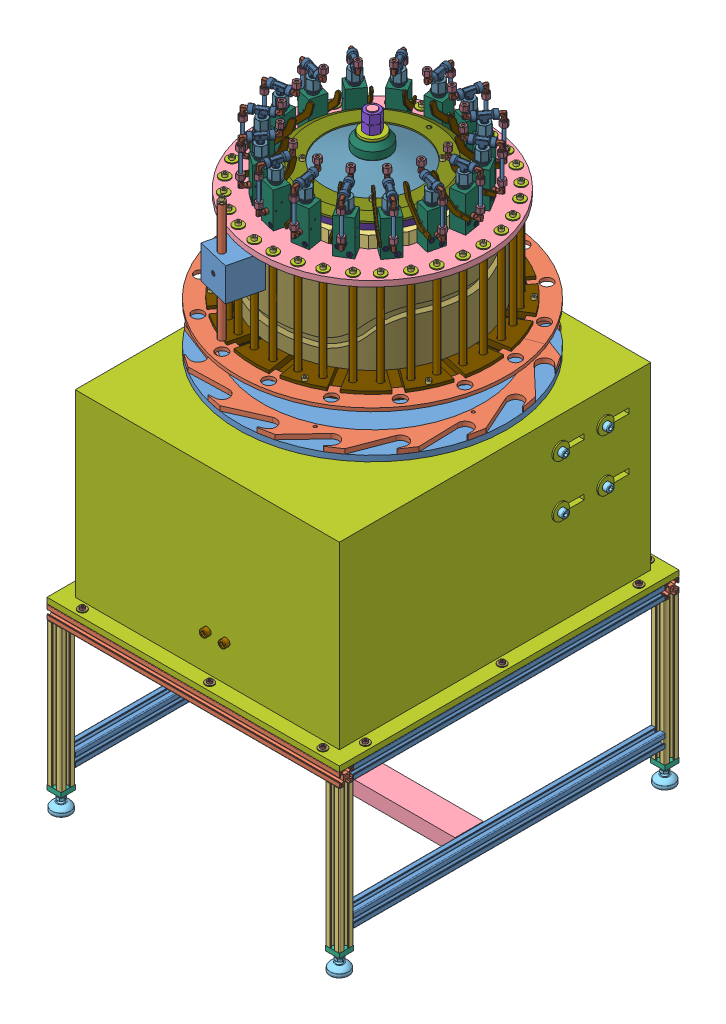
SolidWorks assembly Assieme_FINALE, configuration Default. Lengths in mm. (continued)
Components (placement in the parent): (continued)
- assieme parte rotante-2: assieme parte rotante [Default] at (-8.3038 623.9178 -528.0599) x (0 1 0) z (-0.913062 0 0.407822) size (749.63 778.63 778.63) (continued)
  - AssiemeValvola-14: AssiemeValvola [Default] at (515.3257 186.9093 437.1895) x (0 -0.991445 -0.130526) z (0 -0.130526 0.991445) size (90.26 138.63 38) (continued)
    - LevaValvola-1: LevaValvola [Default] at (-24.507 -86.571 -17) x (0.996193 0.087174 0) z (0 0 1) size (77.55 60.2 4)
    - Tubo-1: Tubo [Default] at (-30 -15.9665 0) x (1 0 0) z (0 -1 0) size (6 6 56.4)
  - AssiemeValvola-15: AssiemeValvola [Default] at (515.3257 182.5711 371.0008) x (0 -0.965926 0.258819) z (0 0.258819 0.965926) size (90.26 138.63 38)
    - RaccordoT-1: RaccordoT [Default] at origin size (43 29.75 16.5)
    - Raccordo a L-1: Raccordo a L [Default] at (-30 0 0) x (0 -1 0) z (0 0 -1) size (28.34 25.51 14.01)
      - 1809_06_10_01-1: 1809_06_10_01 [Default] at origin size (22.49 23 10)
      - 1809_06_10_02-1: 1809_06_10_02 [Default] at origin size (6.5 8.5 8.5)
      - 1809_06_10_03-1: 1809_06_10_03 [Default] at origin size (11.02 15.01 14.01)
    - Raccordo a L-2: Raccordo a L [Default] at (30 0 0) x (0 1 0) z (0 0 -1) size (28.34 25.51 14.01)
      - 1809_06_10_01-1: 1809_06_10_01 [Default] at origin size (22.49 23 10)
      - 1809_06_10_02-1: 1809_06_10_02 [Default] at origin size (6.5 8.5 8.5)
      - 1809_06_10_03-1: 1809_06_10_03 [Default] at origin size (11.02 15.01 14.01)
    - TappoChiusura-1: TappoChiusura [Default] at (0 -32 0) x (0 -1 0) z (0 0 1) size (38.28 26.74 26.74)
    - CorpoValvola-1: CorpoValvola [Default] at (-15 -115.2824 0) size (30 75 34)
    - Raccordo a L-3: Raccordo a L [Default] at (-30 -88.2824 0) x (0 1 0) z (0 0 1) size (28.34 25.51 14.01)
      - 1809_06_10_01-1: 1809_06_10_01 [Default] at origin size (22.49 23 10)
      - 1809_06_10_02-1: 1809_06_10_02 [Default] at origin size (6.5 8.5 8.5)
      - 1809_06_10_03-1: 1809_06_10_03 [Default] at origin size (11.02 15.01 14.01)
    - Spina_3x38-1: Spina_3x38 [Default] at (0 -68.2824 -21) x (-1 0 0) z (0 0 1) size (3 3 38)
    - Spina_3x38-2: Spina_3x38 [Default] at (-10 -80.2824 -21) x (0.996193 0.087174 0) z (0 0 1) size (3 3 38)
    - M5 40mm-3: M5 40mm [ISO 4762 M5 x 40 - 40N] at (-14.6 -108.7824 9) size (45 8.5 8.5)
    - M5 40mm-2: M5 40mm [ISO 4762 M5 x 40 - 40N] at (-14.6 -96.7824 -9) size (45 8.5 8.5)
    - LevaValvola-1: LevaValvola [Default] at (-24.507 -86.571 -17) x (0.996193 0.087174 0) z (0 0 1) size (77.55 60.2 4)
    - Tubo-1: Tubo [Default] at (-30 -15.9665 0) x (1 0 0) z (0 -1 0) size (6 6 56.4)
  - AssiemeValvola-16: AssiemeValvola [Default] at (515.3257 153.2338 311.5106) x (0 -0.793353 0.608761) z (0 0.608761 0.793353) size (90.26 138.63 38)
    - RaccordoT-1: RaccordoT [Default] at origin size (43 29.75 16.5)
    - Raccordo a L-1: Raccordo a L [Default] at (-30 0 0) x (0 -1 0) z (0 0 -1) size (28.34 25.51 14.01)
      - 1809_06_10_01-1: 1809_06_10_01 [Default] at origin size (22.49 23 10)
      - 1809_06_10_02-1: 1809_06_10_02 [Default] at origin size (6.5 8.5 8.5)
      - 1809_06_10_03-1: 1809_06_10_03 [Default] at origin size (11.02 15.01 14.01)
    - Raccordo a L-2: Raccordo a L [Default] at (30 0 0) x (0 1 0) z (0 0 -1) size (28.34 25.51 14.01)
      - 1809_06_10_01-1: 1809_06_10_01 [Default] at origin size (22.49 23 10)
      - 1809_06_10_02-1: 1809_06_10_02 [Default] at origin size (6.5 8.5 8.5)
      - 1809_06_10_03-1: 1809_06_10_03 [Default] at origin size (11.02 15.01 14.01)
    - TappoChiusura-1: TappoChiusura [Default] at (0 -32 0) x (0 -1 0) z (0 0 1) size (38.28 26.74 26.74)
    - CorpoValvola-1: CorpoValvola [Default] at (-15 -115.2824 0) size (30 75 34)
    - Raccordo a L-3: Raccordo a L [Default] at (-30 -88.2824 0) x (0 1 0) z (0 0 1) size (28.34 25.51 14.01)
      - 1809_06_10_01-1: 1809_06_10_01 [Default] at origin size (22.49 23 10)
      - 1809_06_10_02-1: 1809_06_10_02 [Default] at origin size (6.5 8.5 8.5)
      - 1809_06_10_03-1: 1809_06_10_03 [Default] at origin size (11.02 15.01 14.01)
    - Spina_3x38-1: Spina_3x38 [Default] at (0 -68.2824 -21) x (-1 0 0) z (0 0 1) size (3 3 38)
    - Spina_3x38-2: Spina_3x38 [Default] at (-10 -80.2824 -21) x (0.996193 0.087174 0) z (0 0 1) size (3 3 38)
    - M5 40mm-3: M5 40mm [ISO 4762 M5 x 40 - 40N] at (-14.6 -108.7824 9) size (45 8.5 8.5)
    - M5 40mm-2: M5 40mm [ISO 4762 M5 x 40 - 40N] at (-14.6 -96.7824 -9) size (45 8.5 8.5)
    - LevaValvola-1: LevaValvola [Default] at (-24.507 -86.571 -17) x (0.996193 0.087174 0) z (0 0 1) size (77.55 60.2 4)
    - Tubo-1: Tubo [Default] at (-30 -15.9665 0) x (1 0 0) z (0 -1 0) size (6 6 56.4)
  - Disco alimentazione guarnizione fi24.4-1: Disco alimentazione guarnizione fi24.4 [Default] at (198.0433 18.3637 415) x (0 0.065403 0.997859) z (-1 0 0) size (570 285 7.35)
  - Disco alimentazione guarnizione fi24.4-2: Disco alimentazione guarnizione fi24.4 [Default] at (198.0433 18.3637 415) x (0 -0.065403 -0.997859) z (-1 0 0) size (570 285 7.35)
  - m6 12mm-1: m6 12mm [ISO 4762 M6 x 12 - 12N] at (210.0433 200.6849 574.8914) x (-1 0 0) z (0 0.793353 -0.608761) size (18 10 10)
  - m6 12mm-7: m6 12mm [ISO 4762 M6 x 12 - 12N] at (210.0433 260.3445 399.1397) x (-1 0 0) z (0 0.793353 -0.608761) size (18 10 10)
  - m6 12mm-8: m6 12mm [ISO 4762 M6 x 12 - 12N] at (210.0433 96.3128 185.3694) x (-1 0 0) z (0 0.793353 -0.608761) size (18 10 10)
  - m6 12mm-9: m6 12mm [ISO 4762 M6 x 12 - 12N] at (210.0433 -59.5854 644.6306) x (-1 0 0) z (0 -0.793353 -0.608761) size (18 10 10)
  - m6 12mm-10: m6 12mm [ISO 4762 M6 x 12 - 12N] at (210.0433 -223.6171 430.8603) x (-1 0 0) z (0 -0.793353 -0.608761) size (18 10 10)
  - m6 12mm-11: m6 12mm [ISO 4762 M6 x 12 - 12N] at (210.0433 -163.9575 255.1086) x (-1 0 0) z (0 0.793353 -0.608761) size (18 10 10)
- assieme parte fissa-1: assieme parte fissa [Default] at (-1179.2365 708.9757 -309.8267) x (0 -1 0) z (1 0 0) size (784.52 418.9 418.9)
  - AlberoPortaCamme-1: AlberoPortaCamme [Default] at (-462.1354 65.7544 784.523) size (784.52 50 50)
  - linguetta_uni_6604_a_14x9x150-1: linguetta_uni_6604_a_14x9x150 [Default] at (-282.1354 65.7544 802.023) x (1 0 0) z (0 -1 0) size (150 9 14)
  - linguetta_uni_6604_a_8x7x50-1: linguetta_uni_6604_a_8x7x50 [Default] at (-397.1354 65.7544 802.523) x (1 0 0) z (0 1 0) size (50 7 8)
  - linguetta_uni_6604_a_8x7x50-2: linguetta_uni_6604_a_8x7x50 [Default] at (-397.1354 65.7544 766.523) x (1 0 0) z (0 -1 0) size (50 7 8)
  - rondella 20d 50D 5mm-1: rondella 20d 50D 5mm [Default] at (-417.3639 65.7544 784.523) x (0 0 1) z (-1 0 0) size (50 50 5)
  - dado M20-3: dado M20 [ISO - 4034 - M20 - N] at (-441.3639 65.7544 784.523) x (0 -1 0) z (1 0 0) size (30 34.64 19)
  - dado M20-2: dado M20 [ISO - 4034 - M20 - N] at (-422.3639 65.7544 784.523) x (0 -1 0) z (1 0 0) size (30 34.64 19)
  - seger 47-11: seger 47 [B27.7M - 3AM1-50] at (292.1646 65.7544 784.523) x (0 0 -1) z (1 0 0) size (54.93 58.5 1.6)
  - seger 47-12: seger 47 [B27.7M - 3AM1-50] at (272.8646 65.7544 784.523) x (0 0 1) z (-1 0 0) size (54.93 58.5 1.6)
  - seger 47-13: seger 47 [B27.7M - 3AM1-50] at (-120.5354 65.7544 784.523) x (0 0 -1) z (1 0 0) size (54.93 58.5 1.6)
  - seger 47-14: seger 47 [B27.7M - 3AM1-50] at (-104.4354 65.7544 784.523) x (0 0 1) z (-1 0 0) size (54.93 58.5 1.6)
  - seger 45mm-2: seger 45mm [seger 45mm] at (-289.9354 65.7544 784.523) x (0 1 0) z (-1 0 0) size (52.13 56.09 2.8)
  - seger 40mm-3: seger 40mm [B27.8M - 3DM1-40] at (-342.1354 65.7544 784.523) x (0 -1 0) z (1 0 0) size (46.31 50.39 2.8)
  - camma-1: camma [Default] at (-135.1932 65.7544 784.523) x (0 1 0) z (0 0 1) size (418.9 162 418.9)
  - SKF - 6010 - 18,DE,NC,18_68-1: SKF - 6010 - 18,DE,NC,18_68 [SKF - 6010 - 18,DE,NC,18_68] at (282.5646 65.7544 784.523) size (16 80 80)
  - SKF - 6010 - 18,DE,NC,18_68-2: SKF - 6010 - 18,DE,NC,18_68 [SKF - 6010 - 18,DE,NC,18_68] at (-112.5354 65.7544 784.523) size (16 80 80)
  - assieme molla e distributore-2: assieme molla e distributore [Default] at (-388.2308 60.5069 994.523) x (0 -1 0) z (0 0 -1) size (295 75.23 295)
    - molla a tazza-1: molla a tazza [Default] at (-5.2475 5.9046 210) size (200 27.84 200)
    - flangia copertura molla-1: flangia copertura molla [Default] at (-5.2475 11.1331 210) size (70 28.5 70)
    - distributore_fisso-1: distributore_fisso [Default] at (-5.2475 -46.0954 210) x (1 0 0) z (0 1 0) size (295 295 47)
    - delring_distributore_fisso-1: delring_distributore_fisso [Default] at (-5.2475 -46.0954 210) x (0 0 1) z (0 1 0) size (295 295 12)
    - O-ring 12.5x1.8-A-ISO 3601-1-2: O-ring 12.5x1.8-A-ISO 3601-1 [O-ring 12.5x1.8-A-ISO 3601-1] at (-125.2475 -33.1954 210) x (0.868916 0 -0.49496) z (0 1 0) size (16.1 16.1 1.8)
    - M6 16mm-6: M6 16mm [ISO 4762 M6 x 16 - 16N] at (-79.4937 -15.0954 135.7538) x (0 -1 0) z (0 0 1) size (22 10 10)
    - M6 16mm-7: M6 16mm [ISO 4762 M6 x 16 - 16N] at (-79.4937 -15.0954 284.2462) x (0 -1 0) z (1 0 0) size (22 10 10)
    - M6 16mm-8: M6 16mm [ISO 4762 M6 x 16 - 16N] at (68.9987 -15.0954 284.2462) x (0 -1 0) z (0 0 -1) size (22 10 10)
    - M6 16mm-9: M6 16mm [ISO 4762 M6 x 16 - 16N] at (68.9987 -15.0954 135.7538) x (0 -1 0) z (-1 0 0) size (22 10 10)
- assieme_carrello_movimento-1: assieme_carrello_movimento [Default] at (-440.4175 901.0812 -134.2668) x (0.972647 0 0.23229) z (0 1 0) size (70 82 262.71)
  - carello movimento alternativo-1: carello movimento alternativo [Default] at (-11.6011 0.1165 35) size (70 70 70)
  - tubo_carello-1: tubo_carello [Default] at (-11.6011 -19.6699 70) x (0 -1 0) z (0 0 1) size (14 14 250)
  - raccordo dritto-1: raccordo dritto [Default] at (-11.6011 -19.6699 191.1) x (-1 0 0) z (0 1 0) size (14 16.61 13)
  - grano M8 12mm p-1: grano M8 12mm p [ISO 4026 - M8 x 12-N] at (-11.6011 -34.6699 70) x (0 1 0) z (0.714486 0 -0.69965) size (12 8 8)
  - Perno_folle-2: Perno_folle [Default] at (-11.6011 26.4917 70) x (0 1 0) z (0 0 1) size (32 18.94 18.94)
Mates (geometry in assembly coordinates):
- Parallelo2: parallel aligned: plane of SupportoBase_Totale-2 through (4.0127 -14.4529 -3.9361) normal (0 1 0)
- Perpendicolare1: perpendicular: plane of SupportoBase_Totale-2 through (4.0127 -14.4529 -3.9361) normal (0 1 0)
- Parallelo4: parallel aligned: plane of SupportoBase_Totale-2 through (4.0127 -14.4529 -3.9361) normal (0 0 1)
- Coincidente5: coincident anti-aligned: plane of SupportoBase_Totale-2/assieme_base-1/Supporto di Base per macchina-1 through (-154.7135 275.9611 -15.5811) normal (-1 0 0); plane of motoriduttore-1 through (-154.7135 275.9611 -1137.0941) normal (1 0 0)
- Tangente1: tangent anti-aligned: plane of SupportoBase_Totale-2/assieme_base-1/Supporto di Base per macchina-1 through (-93.2286 597.9611 -659.5811) normal (0 1 0); cylinder of motoriduttore-1 through (-154.7135 603.4611 -608.0941) axis (-1 0 0) radius 5.5
- Concentrico1: concentric anti-aligned: cylinder of motoriduttore-1 through (-267.2135 442.7547 -555.0941) axis (0 1 0) radius 15; cylinder of Assieme_Riduttore-1/AlberoRiduttore-1 through (-267.2135 379.4375 -555.0941) axis (0 -1 0) radius 12.5
- Coincidente9: coincident anti-aligned: plane of motoriduttore-1 through (-164.7135 602.1811 -1137.0941) normal (0 1 0); plane of Assieme_Riduttore-1/Rondella di fermo-2 through (-267.2135 602.1811 -555.0941) normal (0 -1 0)
- Coincidente12: coincident anti-aligned: plane of M10 50mm-1 through (-131.7135 606.5159 -520.4879) normal (-1 0 0); plane of plain washer xlarge grade c_iso-1 through (-131.7135 596.9697 -497.3823) normal (1 0 0)
- Concentrico4: concentric aligned: cylinder of M10 50mm-1 through (-89.9635 603.4611 -513.0941) axis (1 0 0) radius 5; cylinder of plain washer xlarge grade c_iso-1 through (-99.7885 603.4611 -513.0941) axis (1 0 0) radius 5.5
- Coincidente13: coincident anti-aligned: plane of M10 50mm-2 through (-131.7135 484.4611 -513.0941) normal (-1 0 0); plane of plain washer xlarge grade c_iso-2 through (-131.7135 475.4611 -513.0941) normal (1 0 0)
- Concentrico5: concentric aligned: cylinder of M10 50mm-2 through (-89.9635 492.4611 -513.0941) axis (1 0 0) radius 5; cylinder of plain washer xlarge grade c_iso-2 through (-99.7885 492.4611 -513.0941) axis (1 0 0) radius 5.5
- Coincidente14: coincident anti-aligned: plane of M10 50mm-5 through (-131.7135 595.4611 -608.0941) normal (-1 0 0); plane of plain washer xlarge grade c_iso-4 through (-131.7135 586.4611 -608.0941) normal (1 0 0)
- Concentrico6: concentric aligned: cylinder of M10 50mm-5 through (-89.9635 603.4611 -608.0941) axis (1 0 0) radius 5; cylinder of plain washer xlarge grade c_iso-4 through (-99.7885 603.4611 -608.0941) axis (1 0 0) radius 5.5
- Coincidente15: coincident anti-aligned: plane of M10 50mm-4 through (-131.7135 484.4611 -608.0941) normal (-1 0 0); plane of plain washer xlarge grade c_iso-3 through (-131.7135 475.4611 -608.0941) normal (1 0 0)
- Concentrico7: concentric aligned: cylinder of M10 50mm-4 through (-89.9635 492.4611 -608.0941) axis (1 0 0) radius 5; cylinder of plain washer xlarge grade c_iso-3 through (-99.7885 492.4611 -608.0941) axis (1 0 0) radius 5.5
- Concentrico8: concentric anti-aligned: cylinder of motoriduttore-1 through (-154.7135 603.4611 -608.0941) axis (-1 0 0) radius 5.5; cylinder of M10 50mm-5 through (-89.9635 603.4611 -608.0941) axis (1 0 0) radius 5
- Coincidente16: coincident anti-aligned: plane of SupportoBase_Totale-2/assieme_base-1/Supporto di Base per macchina-1 through (-134.7135 287.9611 -15.5811) normal (1 0 0); plane of plain washer xlarge grade c_iso-4 through (-134.7135 597.9611 -608.0941) normal (-1 0 0)
- Concentrico9: concentric anti-aligned: cylinder of motoriduttore-1 through (-154.7135 603.4611 -513.0941) axis (-1 0 0) radius 5.5; cylinder of M10 50mm-1 through (-89.9635 603.4611 -513.0941) axis (1 0 0) radius 5
- Coincidente17: coincident anti-aligned: plane of SupportoBase_Totale-2/assieme_base-1/Supporto di Base per macchina-1 through (-134.7135 287.9611 -15.5811) normal (1 0 0); plane of plain washer xlarge grade c_iso-1 through (-134.7135 601.3609 -508.0109) normal (-1 0 0)
- Coincidente18: coincident anti-aligned: plane of SupportoBase_Totale-2/assieme_base-1/Supporto di Base per macchina-1 through (-134.7135 287.9611 -15.5811) normal (1 0 0); plane of plain washer xlarge grade c_iso-3 through (-134.7135 486.9611 -608.0941) normal (-1 0 0)
- Concentrico10: concentric aligned: circle of motoriduttore-1; cylinder of M10 50mm-4 through (-89.9635 492.4611 -608.0941) axis (1 0 0) radius 5
- Coincidente19: coincident anti-aligned: plane of SupportoBase_Totale-2/assieme_base-1/Supporto di Base per macchina-1 through (-134.7135 287.9611 -15.5811) normal (1 0 0); plane of plain washer xlarge grade c_iso-2 through (-134.7135 486.9611 -513.0941) normal (-1 0 0)
- Concentrico11: concentric aligned: circle of motoriduttore-1; cylinder of M10 50mm-2 through (-89.9635 492.4611 -513.0941) axis (1 0 0) radius 5
- Concentrico12: concentric anti-aligned: cylinder of M10 50mm-4 through (-89.9635 492.4611 -608.0941) axis (1 0 0) radius 5; cylinder of hex nut style 2 gradeab_iso-7 through (-164.7135 492.4611 -608.0941) axis (-1 0 0) radius 4.25
- Coincidente20: coincident anti-aligned: plane of motoriduttore-1 through (-164.7135 275.9611 -1137.0941) normal (-1 0 0); plane of hex nut style 2 gradeab_iso-7 through (-164.7135 501.6987 -608.0941) normal (1 0 0)
- Concentrico13: concentric anti-aligned: cylinder of M10 50mm-5 through (-89.9635 603.4611 -608.0941) axis (1 0 0) radius 5; cylinder of hex nut style 2 gradeab_iso-5 through (-164.7135 603.4611 -608.0941) axis (-1 0 0) radius 4.25
- Coincidente21: coincident aligned: plane of motoriduttore-1 through (-164.7135 275.9611 -1137.0941) normal (-1 0 0); circle of hex nut style 2 gradeab_iso-1
- Concentrico14: concentric anti-aligned: cylinder of M10 50mm-1 through (-89.9635 603.4611 -513.0941) axis (1 0 0) radius 5; cylinder of hex nut style 2 gradeab_iso-8 through (-164.7135 603.4611 -513.0941) axis (-1 0 0) radius 4.25
- Coincidente22: coincident anti-aligned: plane of motoriduttore-1 through (-164.7135 275.9611 -1137.0941) normal (-1 0 0); plane of hex nut style 2 gradeab_iso-8 through (-164.7135 612.6987 -513.0941) normal (1 0 0)
- Concentrico15: concentric anti-aligned: cylinder of M10 50mm-2 through (-89.9635 492.4611 -513.0941) axis (1 0 0) radius 5; cylinder of hex nut style 2 gradeab_iso-6 through (-164.7135 492.4611 -513.0941) axis (-1 0 0) radius 4.25
- Coincidente23: coincident anti-aligned: plane of motoriduttore-1 through (-164.7135 275.9611 -1137.0941) normal (-1 0 0); plane of hex nut style 2 gradeab_iso-6 through (-164.7135 501.6987 -513.0941) normal (1 0 0)
- Concentrico164: concentric anti-aligned: cylinder of SupportoBase_Totale-2/assieme_base-1/Traversa di blocco albero-1 through (-394.7135 362.1119 -360.5811) axis (0 1 0) radius 5.25; cylinder of assieme parte fissa-1/AlberoPortaCamme-1 through (-394.7135 386.9611 -360.5811) axis (0 -1 0) radius 4.5
- Coincidente26: coincident anti-aligned: plane of SupportoBase_Totale-2/assieme_base-1/Traversa di blocco albero-1 through (-427.2135 386.9611 -53.5811) normal (0 1 0); plane of assieme parte fissa-1/AlberoPortaCamme-1 through (-394.7135 386.9611 -400.5811) normal (0 -1 0)
- Concentrico1651: concentric aligned: cylinder of SupportoBase_Totale-2/assieme_base-1/Traversa di blocco albero-1 through (-394.7135 362.1119 -360.5811) axis (0 1 0) radius 5.25; cylinder of rondella M8-1 through (-394.7135 374.9611 -360.5811) axis (0 1 0) radius 4.65
- Coincidente271: coincident anti-aligned: plane of SupportoBase_Totale-2/assieme_base-1/Traversa di blocco albero-1 through (-427.2135 376.9611 -53.5811) normal (0 -1 0); plane of rondella M8-1 through (-394.7135 376.9611 -360.5811) normal (0 1 0)
- Concentrico1661: concentric aligned: cylinder of SupportoBase_Totale-2/assieme_base-1/Traversa di blocco albero-1 through (-394.7135 362.1119 -390.5811) axis (0 1 0) radius 5.25; cylinder of rondella M8-2 through (-394.7135 374.9611 -390.5811) axis (0 1 0) radius 4.65
- Coincidente281: coincident anti-aligned: plane of SupportoBase_Totale-2/assieme_base-1/Traversa di blocco albero-1 through (-427.2135 376.9611 -53.5811) normal (0 -1 0); plane of rondella M8-2 through (-394.7135 376.9611 -390.5811) normal (0 1 0)
- Coincidente29: coincident aligned: plane of rondella M8-1 through (-394.7135 376.9611 -360.5811) normal (-1 0 0); plane of rondella M8-2 through (-394.7135 376.9611 -390.5811) normal (-1 0 0)
- Concentrico16621: concentric anti-aligned: cylinder of SupportoBase_Totale-2/assieme_base-1/Traversa di blocco albero-1 through (-394.7135 362.1119 -390.5811) axis (0 1 0) radius 5.25; cylinder of M8 25 mm-1 through (-394.7135 337.2111 -390.5811) axis (0 -1 0) radius 6.5
- Coincidente2821: coincident anti-aligned: plane of SupportoBase_Totale-2/assieme_base-1/Traversa di blocco albero-1 through (-427.2135 376.9611 -53.5811) normal (0 -1 0); plane of M8 25 mm-1 through (-400.3427 376.9611 -387.3311) normal (0 1 0)
- Concentrico16631: concentric anti-aligned: cylinder of rondella M8-1 through (-394.7135 374.9611 -360.5811) axis (0 1 0) radius 4.65; cylinder of M8 25 mm-2 through (-394.7135 335.2111 -360.5811) axis (0 -1 0) radius 6.5
- Coincidente284: coincident anti-aligned: plane of rondella M8-1 through (-394.7135 374.9611 -360.5811) normal (0 -1 0); plane of M8 25 mm-2 through (-389.0844 374.9611 -363.8311) normal (0 1 0)
- Coincidente285: coincident aligned: plane of M8 25 mm-1 through (-391.666 372.9611 -388.8216) normal (-1 0 0); plane of M8 25 mm-2 through (-391.666 370.9611 -362.3406) normal (-1 0 0)
- Concentrico16632: concentric aligned: cylinder of assieme parte rotante-1/asta scorrimento carello-15 through (-613.1413 1023.9611 -329.7302) axis (0 -1 0) radius 6; cylinder of assieme_carrello_movimento-1/carello movimento alternativo-1 through (-423.911 1006.0812 -154.3109) axis (0 -1 0) radius 7
- Concentrico16635: concentric anti-aligned: cylinder of assieme parte rotante-1/asta scorrimento carello-30 through (-617.9018 798.9611 -375.4832) axis (0 1 0) radius 6; cylinder of assieme_carrello_movimento-1/carello movimento alternativo-1 through (-468.6528 1006.0812 -164.9962) axis (0 -1 0) radius 7
- Concentrico16648: concentric aligned: cylinder of assieme parte fissa-1/AlberoPortaCamme-1 through (-394.7135 1275.1556 -375.5811) axis (0 1 0) radius 25; cylinder of assieme parte rotante-2/albero rotazione piatti-1 through (-394.7135 684.3308 -375.5811) axis (0 1 0) radius 35
- Coincidente2822: coincident anti-aligned: plane of SupportoBase_Totale-2/assieme_base-1/canotto di supporto-1 through (-394.7135 673.9611 -375.5811) normal (0 1 0); plane of assieme parte rotante-2/SKF - 6020 - 20,DE,NC,20_68-2 through (-396.2853 673.9611 -318.1026) normal (0 -1 0)
- Concentrico16650: concentric aligned: cylinder of SupportoBase_Totale-2/assieme_base-1/canotto di supporto-1 through (-394.7135 587.1745 -375.5811) axis (0 1 0) radius 67.5; cylinder of assieme parte fissa-1/AlberoPortaCamme-1 through (-394.7135 1275.1556 -375.5811) axis (0 1 0) radius 25
- Concentrico16651: concentric anti-aligned: cylinder of assieme parte rotante-2/asta scorrimento carello-23 through (-468.6528 798.9611 -164.9962) axis (0 1 0) radius 6; cylinder of assieme_carrello_movimento-1/carello movimento alternativo-1 through (-468.6528 1006.0812 -164.9962) axis (0 -1 0) radius 7
- Concentrico16652: concentric aligned: cylinder of assieme parte rotante-2/asta scorrimento carello-8 through (-423.911 1023.9611 -154.3109) axis (0 -1 0) radius 6; cylinder of assieme_carrello_movimento-1/carello movimento alternativo-1 through (-423.911 1006.0812 -154.3109) axis (0 -1 0) radius 7
- Tangente8: tangent: face of assieme parte fissa-1/camma-1; cylinder of ? through (-185.8875 941.1413 -276.1155) axis (0.902819 0 0.430021) radius 9.47
